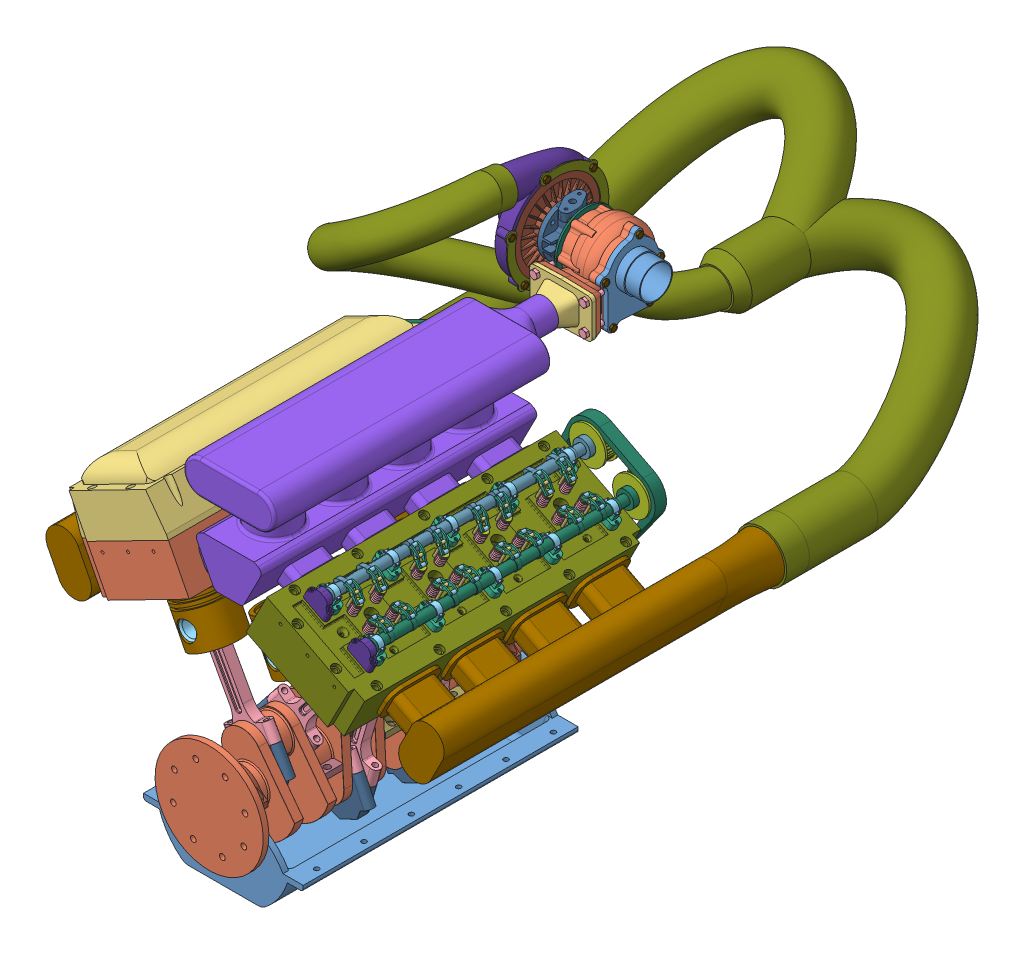
SolidWorks assembly ENSAMBLAJE DE MOTOR V8, configuration Predeterminado. Lengths in mm. (continued)
Mates (geometry in assembly coordinates): (continued)
- Distancia límite16: limit distance = 1.2344 mm: cone of assembly; cone of assembly; cone of CULATA_IZQUIERDO-2 through (128.2013 136.8296 302.75) axis (0.455744 0.890111 0); cone of VÁLVULA-18 through (127.4565 135.3748 302.75) axis (0.455744 0.890111 0)
- Concéntrica175: concentric: cylinder of assembly; cylinder of assembly; cylinder of CULATA_DERECHO-1 through (-129.9528 150.5383 696.25) axis (-0.455744 0.890111 0) radius 3; cylinder of VÁLVULA-1 through (-129.448 149.5524 696.25) axis (0.455744 -0.890111 0) radius 3
- Distancia límite13: limit distance = 0 mm: plane of assembly; plane of assembly; plane of CULATA_DERECHO-1 through (-140.7516 143.3241 454.25) normal (0.455744 -0.890111 0); plane of VÁLVULA-14 through (-155.9725 135.5309 434.25) normal (0.455744 -0.890111 0)
- Coincidente89: coincident: plane of assembly; plane of assembly; plane of RESORTE DE VÁLVULA-1 through (-174.795 238.1196 696.25) normal (-0.455744 0.890111 0); plane of VÁLVULA-1 through (-174.795 238.1196 696.25) normal (0.455744 -0.890111 0)
- Concéntrica176: concentric: cylinder of assembly; cylinder of assembly; cylinder of RESORTE DE VÁLVULA-1 through (-173.7217 236.0234 696.25) axis (-0.455744 0.890111 0) radius 7.3; cylinder of VÁLVULA-1 through (-129.448 149.5524 696.25) axis (0.455744 -0.890111 0) radius 3
- Distancia límite1: limit distance = 0.0087 mm: cone of assembly; cone of assembly; cone of CULATA_DERECHO-1 through (-129.9528 150.5383 696.25) axis (-0.455744 0.890111 0); cone of VÁLVULA-1 through (-129.2657 149.1964 696.25) axis (-0.455744 0.890111 0)
- Coincidente90: coincident: circle of CULATA_DERECHO-1; plane of ? through (-149.3077 210.2827 694) normal (0.455744 -0.890111 0)
- Concéntrica177: concentric: cylinder of CULATA_DERECHO-1 through (-156.1439 223.6343 696.25) axis (-0.455744 0.890111 0) radius 2.25; cylinder of ? through (-149.3077 210.2827 696.25) axis (0.455744 -0.890111 0) radius 2.25
- Paralelo3: parallel: plane of assembly; plane of assembly; plane of ARBOL DE LEVAS DE ADMISIÓN_DERECHO-1 through (-136.0099 236.5757 692.45) normal (0 0 -1); plane of EJE DE CONTROL DE VÁLVULAS-1 through (-180.6988 240.2228 703.25) normal (0 0 1)
- Paralelo4: parallel: plane of assembly; plane of assembly; plane of EJE DE CONTROL DE VÁLVULAS-1 through (-180.6988 240.2228 689.25) normal (0 0 -1); plane of RESORTE DE VÁLVULA-1 through (-160.667 210.5262 703.4) normal (0 0 1)
- Concéntrica178: concentric: cylinder of assembly; cylinder of assembly; cylinder of EJE DE CONTROL DE VÁLVULAS-1 through (-180.6988 240.2228 703.25) axis (0 0 -1) radius 2.5; cylinder of SOPORTE DE SEGUIDOR DE VÁLVULA-1 through (-180.6988 240.2228 691.95) axis (0 0 -1) radius 2.5
- Concéntrica179: concentric: cylinder of assembly; cylinder of assembly; cylinder of SOPORTE DE SEGUIDOR DE VÁLVULA-1 through (-191.9772 233.816 700.55) axis (0 0 -1) radius 1.9; cylinder of SEGUIDOR DE LEVA-13 through (-191.9772 233.816 700.05) axis (0 0 -1) radius 3
- Ancho17: width: plane of assembly; plane of assembly; plane of assembly; plane of assembly; plane of EJE DE CONTROL DE VÁLVULAS-1 through (-180.6988 240.2228 689.25) normal (0 0 -1); plane of EJE DE CONTROL DE VÁLVULAS-1 through (-180.6988 240.2228 703.25) normal (0 0 1); plane of SOPORTE DE SEGUIDOR DE VÁLVULA-1 through (-189.0856 245.1951 691.95) normal (0 0 1); plane of SOPORTE DE SEGUIDOR DE VÁLVULA-1 through (-176.0253 239.3734 700.55) normal (0 0 -1)
- Ancho18: width: plane of assembly; plane of assembly; plane of assembly; plane of assembly; plane of SOPORTE DE SEGUIDOR DE VÁLVULA-1 through (-176.0253 239.3734 700.55) normal (0 0 -1); plane of SOPORTE DE SEGUIDOR DE VÁLVULA-1 through (-189.0856 245.1951 691.95) normal (0 0 1); plane of SEGUIDOR DE LEVA-13 through (-191.9772 233.816 692.45) normal (0 0 -1); plane of SEGUIDOR DE LEVA-13 through (-191.9772 233.816 700.05) normal (0 0 1)
- Concéntrica181: concentric: cylinder of assembly; cylinder of assembly; cylinder of SEGUIDOR DE LEVA-1 through (-166.3151 243.7387 700.05) axis (0 0 -1) radius 3; cylinder of SOPORTE DE SEGUIDOR DE VÁLVULA-1 through (-166.3151 243.7387 700.55) axis (0 0 -1) radius 1.9
- Ancho19: width: plane of assembly; plane of assembly; plane of assembly; plane of assembly; plane of SOPORTE DE SEGUIDOR DE VÁLVULA-1 through (-189.0856 245.1951 689.45) normal (0 0 -1); plane of SOPORTE DE SEGUIDOR DE VÁLVULA-1 through (-176.0253 239.3734 703.05) normal (0 0 1); plane of SEGUIDOR DE LEVA-1 through (-166.3151 243.7387 700.05) normal (0 0 1); plane of SEGUIDOR DE LEVA-1 through (-166.3151 243.7387 692.45) normal (0 0 -1)
- Tangente3: tangent: plane of assembly; cylinder of assembly; plane of VÁLVULA-1 through (-175.2508 239.0097 696.25) normal (-0.455744 0.890111 0); cylinder of SEGUIDOR DE LEVA-13 through (-191.9772 233.816 700.05) axis (0 0 -1) radius 3
- Relación de posición de Leva Tangente1: cam tangent: cylinder of ARBOL DE LEVAS DE ADMISIÓN_DERECHO-1 through (-159.0489 247.0856 692.45) axis (0 0 1) radius 5; cylinder of SEGUIDOR DE LEVA-1 through (-166.3151 243.7387 700.05) axis (0 0 -1) radius 3
- Concéntrica182: concentric: cylinder of assembly; cylinder of assembly; cylinder of SOPORTE DE SEGUIDOR DE VÁLVULA-2 through (-177.5936 240.5206 588.55) axis (0 0 -1) radius 1.9; cylinder of SEGUIDOR DE LEVA-21 through (-177.5936 240.5206 588.05) axis (0 0 -1) radius 3
- Concéntrica183: concentric: cylinder of assembly; cylinder of assembly; cylinder of EJE DE CONTROL DE VÁLVULAS-2 through (-170.2719 251.2278 591.25) axis (0 0 -1) radius 2.5; cylinder of SOPORTE DE SEGUIDOR DE VÁLVULA-2 through (-170.2719 251.2278 579.95) axis (0 0 -1) radius 2.5
- Concéntrica184: concentric: cylinder of assembly; cylinder of assembly; cylinder of RESORTE DE VÁLVULA-2 through (-173.454 235.5005 584.25) axis (-0.455744 0.890111 0) radius 7.3; cylinder of VÁLVULA-2 through (-129.1802 149.0296 584.25) axis (0.455744 -0.890111 0) radius 3
- Ancho20: width: plane of SOPORTE DE SEGUIDOR DE VÁLVULA-2 through (-179.9902 252.0141 577.45) normal (0 0 -1); plane of SOPORTE DE SEGUIDOR DE VÁLVULA-2 through (-165.6999 252.5159 591.05) normal (0 0 1); plane of SEGUIDOR DE LEVA-17 through (-158.8913 260.7004 588.05) normal (0 0 1); plane of SEGUIDOR DE LEVA-17 through (-158.8913 260.7004 580.45) normal (0 0 -1)
- Ancho21: width: plane of assembly; plane of assembly; plane of assembly; plane of assembly; plane of EJE DE CONTROL DE VÁLVULAS-2 through (-170.2719 251.2278 577.25) normal (0 0 -1); plane of EJE DE CONTROL DE VÁLVULAS-2 through (-170.2719 251.2278 591.25) normal (0 0 1); plane of SOPORTE DE SEGUIDOR DE VÁLVULA-2 through (-179.9902 252.0141 579.95) normal (0 0 1); plane of SOPORTE DE SEGUIDOR DE VÁLVULA-2 through (-165.6999 252.5159 588.55) normal (0 0 -1)
- Concéntrica185: concentric: cylinder of SEGUIDOR DE LEVA-17 through (-158.8913 260.7004 588.05) axis (0 0 -1) radius 3; cylinder of SOPORTE DE SEGUIDOR DE VÁLVULA-2 through (-158.8913 260.7004 588.55) axis (0 0 -1) radius 1.9
- Tangente4: tangent: plane of assembly; cylinder of assembly; plane of VÁLVULA-2 through (-174.983 238.4868 584.25) normal (-0.455744 0.890111 0); cylinder of SEGUIDOR DE LEVA-21 through (-177.5936 240.5206 588.05) axis (0 0 -1) radius 3
- Paralelo5: parallel: plane of assembly; plane of assembly; plane of EJE DE CONTROL DE VÁLVULAS-2 through (-170.2719 251.2278 577.25) normal (0 0 -1); plane of RESORTE DE VÁLVULA-2 through (-160.3993 210.0033 591.4) normal (0 0 1)
- Ancho22: width: plane of assembly; plane of assembly; plane of assembly; plane of assembly; plane of SOPORTE DE SEGUIDOR DE VÁLVULA-2 through (-165.6999 252.5159 588.55) normal (0 0 -1); plane of SOPORTE DE SEGUIDOR DE VÁLVULA-2 through (-179.9902 252.0141 579.95) normal (0 0 1); plane of SEGUIDOR DE LEVA-21 through (-177.5936 240.5206 580.45) normal (0 0 -1); plane of SEGUIDOR DE LEVA-21 through (-177.5936 240.5206 588.05) normal (0 0 1)
- Coincidente93: coincident: plane of assembly; plane of assembly; plane of RESORTE DE VÁLVULA-2 through (-174.5273 237.5967 584.25) normal (-0.455744 0.890111 0); plane of VÁLVULA-2 through (-174.5273 237.5967 584.25) normal (0.455744 -0.890111 0)
- Coincidente94: coincident: circle of assembly; plane of assembly; circle of CULATA_DERECHO-1; plane of EJE DE CONTROL DE VÁLVULAS-2 through (-149.3077 210.2827 582) normal (0.455744 -0.890111 0)
- Concéntrica186: concentric: cylinder of assembly; cylinder of assembly; cylinder of CULATA_DERECHO-1 through (-129.9528 150.5383 584.25) axis (-0.455744 0.890111 0) radius 3; cylinder of VÁLVULA-2 through (-129.1802 149.0296 584.25) axis (0.455744 -0.890111 0) radius 3
- Distancia límite2: limit distance = 1.6951 mm: plane of assembly; plane of assembly; plane of CULATA_DERECHO-1 through (-140.7516 143.3241 564.25) normal (0.455744 -0.890111 0); plane of VÁLVULA-2 through (-128.4966 147.6944 584.25) normal (0.455744 -0.890111 0)
- Concéntrica187: concentric: cylinder of assembly; cylinder of assembly; cylinder of CULATA_DERECHO-1 through (-156.1439 223.6343 584.25) axis (-0.455744 0.890111 0) radius 2.25; cylinder of EJE DE CONTROL DE VÁLVULAS-2 through (-149.3077 210.2827 584.25) axis (0.455744 -0.890111 0) radius 2.25
- Paralelo6: parallel: plane of assembly; plane of assembly; plane of RESORTE DE VÁLVULA-2 through (-160.3993 210.0033 577.1) normal (0 0 -1); plane of SOPORTE DE SEGUIDOR DE VÁLVULA-2 through (-179.9902 252.0141 577.45) normal (0 0 -1)
- Relación de posición de Leva Tangente2: cam tangent: cylinder of ARBOL DE LEVAS DE ADMISIÓN_DERECHO-1 through (-150.1483 251.4202 588.05) axis (0 0 -1) radius 9.75; cylinder of SEGUIDOR DE LEVA-17 through (-158.8913 260.7004 588.05) axis (0 0 -1) radius 3
- Paralelo9: parallel: plane of assembly; plane of assembly; plane of ARBOL DE LEVAS DE ADMISIÓN_DERECHO-1 through (-170.2396 250.2568 588.05) normal (0 0 1); plane of SOPORTE DE SEGUIDOR DE VÁLVULA-2 through (-165.6999 252.5159 591.05) normal (0 0 1)
- Distancia límite4: limit distance = 1.1076 mm: plane of assembly; plane of assembly; plane of CULATA_DERECHO-1 through (-140.7516 143.3241 676.25) normal (0.455744 -0.890111 0); plane of VÁLVULA-3 through (-128.7643 148.2172 656.25) normal (0.455744 -0.890111 0)
- Distancia límite5: limit distance = 1.6951 mm: plane of assembly; plane of assembly; plane of CULATA_DERECHO-1 through (-140.7516 143.3241 564.25) normal (0.455744 -0.890111 0); plane of VÁLVULA-4 through (-128.4966 147.6944 544.25) normal (0.455744 -0.890111 0)
- Distancia límite6: limit distance = 1.1076 mm: plane of assembly; plane of assembly; plane of CULATA_DERECHO-1 through (-140.7516 143.3241 344.25) normal (0.455744 -0.890111 0); plane of VÁLVULA-6 through (-128.7643 148.2172 324.25) normal (0.455744 -0.890111 0)
- Distancia límite7: limit distance = 1.1076 mm: plane of assembly; plane of assembly; plane of CULATA_DERECHO-1 through (-140.7516 143.3241 344.25) normal (0.455744 -0.890111 0); plane of VÁLVULA-5 through (-128.7643 148.2172 364.25) normal (0.455744 -0.890111 0)
- Concéntrica189: concentric: cylinder of assembly; cylinder of assembly; cylinder of RESORTE DE VÁLVULA-9 through (-200.4251 222.3511 696.25) axis (-0.455744 0.890111 0) radius 7.3; cylinder of VÁLVULA-9 through (-156.1513 135.8801 696.25) axis (0.455744 -0.890111 0) radius 3
- Coincidente96: coincident: plane of RESORTE DE VÁLVULA-9 through (-201.4983 224.4473 696.25) normal (-0.455744 0.890111 0); plane of VÁLVULA-9 through (-201.4983 224.4473 696.25) normal (0.455744 -0.890111 0)
- Concéntrica190: concentric: cylinder of CULATA_DERECHO-1 through (-156.6561 136.866 696.25) axis (-0.455744 0.890111 0) radius 3; cylinder of VÁLVULA-9 through (-156.1513 135.8801 696.25) axis (0.455744 -0.890111 0) radius 3
- Distancia límite8: limit distance = 1.1076 mm: plane of CULATA_DERECHO-1 through (-140.7516 143.3241 676.25) normal (0.455744 -0.890111 0); plane of VÁLVULA-9 through (-155.4677 134.5449 696.25) normal (0.455744 -0.890111 0)
- Concéntrica191: concentric: cylinder of assembly; cylinder of assembly; cylinder of EJE DE CONTROL DE VÁLVULAS-9 through (-214.7775 228.4406 689.25) axis (0 0 1) radius 2.5; cylinder of SOPORTE DE SEGUIDOR DE VÁLVULA-9 through (-214.7775 228.4406 700.55) axis (0 0 1) radius 2.5
- Concéntrica192: concentric: cylinder of SEGUIDOR DE LEVA-25 through (-201.8109 228.7811 692.45) axis (0 0 1) radius 3; cylinder of SOPORTE DE SEGUIDOR DE VÁLVULA-9 through (-201.8109 228.7811 691.95) axis (0 0 1) radius 1.9
- Concéntrica193: concentric: cylinder of SOPORTE DE SEGUIDOR DE VÁLVULA-9 through (-228.9095 224.0206 691.95) axis (0 0 1) radius 1.9; cylinder of SEGUIDOR DE LEVA-34 through (-228.9095 224.0206 692.45) axis (0 0 1) radius 3
- Ancho24: width: plane of SOPORTE DE SEGUIDOR DE VÁLVULA-9 through (-210.1649 237.0305 703.05) normal (0 0 1); plane of SOPORTE DE SEGUIDOR DE VÁLVULA-9 through (-218.3403 225.299 689.45) normal (0 0 -1); plane of SEGUIDOR DE LEVA-34 through (-228.9095 224.0206 692.45) normal (0 0 -1); plane of SEGUIDOR DE LEVA-34 through (-228.9095 224.0206 700.05) normal (0 0 1)
- Ancho25: width: plane of SOPORTE DE SEGUIDOR DE VÁLVULA-9 through (-210.1649 237.0305 703.05) normal (0 0 1); plane of SOPORTE DE SEGUIDOR DE VÁLVULA-9 through (-218.3403 225.299 689.45) normal (0 0 -1); plane of EJE DE CONTROL DE VÁLVULAS-9 through (-214.7775 228.4406 703.25) normal (0 0 1); plane of EJE DE CONTROL DE VÁLVULAS-9 through (-214.7775 228.4406 689.25) normal (0 0 -1)
- Ancho26: width: plane of SEGUIDOR DE LEVA-25 through (-201.8109 228.7811 700.05) normal (0 0 1); plane of SEGUIDOR DE LEVA-25 through (-201.8109 228.7811 692.45) normal (0 0 -1); plane of SOPORTE DE SEGUIDOR DE VÁLVULA-9 through (-218.3403 225.299 689.45) normal (0 0 -1); plane of SOPORTE DE SEGUIDOR DE VÁLVULA-9 through (-210.1649 237.0305 703.05) normal (0 0 1)
- Concéntrica194: concentric: cylinder of assembly; cylinder of assembly; cylinder of RESORTE DE VÁLVULA-10 through (-190.6415 203.2427 584.25) axis (-0.455744 0.890111 0) radius 5.25; cylinder of VÁLVULA-10 through (-156.6561 136.866 584.25) axis (0.455744 -0.890111 0) radius 3
- Concéntrica195: concentric: cylinder of assembly; cylinder of assembly; cylinder of SEGUIDOR DE LEVA-38 through (-228.4393 222.7305 580.45) axis (0 0 1) radius 3; cylinder of SOPORTE DE SEGUIDOR DE VÁLVULA-10 through (-228.4393 222.7305 579.95) axis (0 0 1) radius 1.9
- Concéntrica196: concentric: cylinder of EJE DE CONTROL DE VÁLVULAS-10 through (-214.7775 228.4406 591.25) axis (0 0 -1) radius 2.5; cylinder of SOPORTE DE SEGUIDOR DE VÁLVULA-10 through (-214.7775 228.4406 577.45) axis (0 0 1) radius 2.5
- Concéntrica197: concentric: cylinder of CULATA_DERECHO-1 through (-200.6495 200.8471 584.25) axis (-0.455744 0.890111 0) radius 2.25; cylinder of EJE DE CONTROL DE VÁLVULAS-10 through (-193.8133 187.4955 584.25) axis (0.455744 -0.890111 0) radius 2.25
- Ancho27: width: plane of SOPORTE DE SEGUIDOR DE VÁLVULA-10 through (-210.9805 237.4209 588.55) normal (0 0 -1); plane of SOPORTE DE SEGUIDOR DE VÁLVULA-10 through (-218.0339 224.9825 579.95) normal (0 0 1); plane of EJE DE CONTROL DE VÁLVULAS-10 through (-214.7775 228.4406 591.25) normal (0 0 1); plane of EJE DE CONTROL DE VÁLVULAS-10 through (-214.7775 228.4406 577.25) normal (0 0 -1)
- Coincidente100: coincident: circle of CULATA_DERECHO-1; plane of EJE DE CONTROL DE VÁLVULAS-10 through (-193.8133 187.4955 582) normal (0.455744 -0.890111 0)
- Ancho28: width: plane of ARBOL DE LEVAS DE ESCAPE_DERECHO-1 through (-245.4839 205.0082 580.45) normal (0 0 -1); plane of ARBOL DE LEVAS DE ESCAPE_DERECHO-1 through (-245.4839 205.0082 588.05) normal (0 0 1); plane of EJE DE CONTROL DE VÁLVULAS-10 through (-214.7775 228.4406 591.25) normal (0 0 1); plane of EJE DE CONTROL DE VÁLVULAS-10 through (-214.7775 228.4406 577.25) normal (0 0 -1)
- Ancho29: width: plane of SEGUIDOR DE LEVA-38 through (-228.4393 222.7305 588.05) normal (0 0 1); plane of SEGUIDOR DE LEVA-38 through (-228.4393 222.7305 580.45) normal (0 0 -1); plane of SOPORTE DE SEGUIDOR DE VÁLVULA-10 through (-218.0339 224.9825 577.45) normal (0 0 -1); plane of SOPORTE DE SEGUIDOR DE VÁLVULA-10 through (-210.9805 237.4209 591.05) normal (0 0 1)
- Concéntrica198: concentric: cylinder of assembly; cylinder of assembly; cylinder of CULATA_DERECHO-1 through (-187.1909 196.5035 584.25) axis (-0.455744 0.890111 0) radius 7.3; cylinder of VÁLVULA-10 through (-156.6561 136.866 584.25) axis (0.455744 -0.890111 0) radius 3
- Coincidente101: coincident: plane of RESORTE DE VÁLVULA-10 through (-202.0031 225.4332 584.25) normal (-0.455744 0.890111 0); plane of VÁLVULA-10 through (-202.0031 225.4332 584.25) normal (0.455744 -0.890111 0)
- Concéntrica199: concentric: cylinder of SOPORTE DE SEGUIDOR DE VÁLVULA-10 through (-201.8981 229.9808 579.95) axis (0 0 1) radius 1.9; cylinder of SEGUIDOR DE LEVA-42 through (-201.8981 229.9808 588.05) axis (0 0 -1) radius 1.9
- Ancho30: width: plane of SEGUIDOR DE LEVA-42 through (-201.8981 229.9808 588.05) normal (0 0 1); plane of SEGUIDOR DE LEVA-42 through (-201.8981 229.9808 580.45) normal (0 0 -1); plane of SOPORTE DE SEGUIDOR DE VÁLVULA-10 through (-210.9805 237.4209 591.05) normal (0 0 1); plane of SOPORTE DE SEGUIDOR DE VÁLVULA-10 through (-218.0339 224.9825 577.45) normal (0 0 -1)
- Tangente6: tangent: plane of VÁLVULA-10 through (-202.4589 226.3233 584.25) normal (-0.455744 0.890111 0); cylinder of SEGUIDOR DE LEVA-42 through (-201.8981 229.9808 588.05) axis (0 0 -1) radius 3
- Distancia límite10: limit distance = 1.1076 mm: plane of assembly; plane of assembly; plane of CULATA_DERECHO-1 through (-140.7516 143.3241 676.25) normal (0.455744 -0.890111 0); plane of VÁLVULA-11 through (-155.4677 134.5449 656.25) normal (0.455744 -0.890111 0)
- Distancia límite14: limit distance = 1.1076 mm: plane of assembly; plane of assembly; plane of CULATA_DERECHO-1 through (-140.7516 143.3241 344.25) normal (0.455744 -0.890111 0); plane of VÁLVULA-15 through (-155.4677 134.5449 364.25) normal (0.455744 -0.890111 0)
- Distancia límite15: limit distance = 1.1076 mm: plane of assembly; plane of assembly; plane of CULATA_DERECHO-1 through (-140.7516 143.3241 344.25) normal (0.455744 -0.890111 0); plane of VÁLVULA-16 through (-155.4677 134.5449 324.25) normal (0.455744 -0.890111 0)
- Concéntrica201: concentric: cylinder of assembly; cylinder of assembly; cylinder of CULATA_IZQUIERDO-2 through (172.1947 200.8107 302.75) axis (0.455744 0.890111 0) radius 2.25; cylinder of EJE DE CONTROL DE VÁLVULAS-17 through (165.3585 187.459 302.75) axis (-0.455744 -0.890111 0) radius 2.25
- Concéntrica202: concentric: cylinder of assembly; cylinder of assembly; cylinder of RESORTE DE VÁLVULA-17 through (161.6241 202.1075 302.75) axis (0.455744 0.890111 0) radius 5.25; cylinder of VÁLVULA-18 through (127.6388 135.7308 302.75) axis (-0.455744 -0.890111 0) radius 3
- Coincidente103: coincident: plane of RESORTE DE VÁLVULA-17 through (172.9858 224.298 302.75) normal (0.455744 0.890111 0); plane of VÁLVULA-18 through (172.9858 224.298 302.75) normal (-0.455744 -0.890111 0)
- Concéntrica203: concentric: cylinder of assembly; cylinder of assembly; cylinder of CULATA_IZQUIERDO-2 through (128.2013 136.8296 302.75) axis (0.455744 0.890111 0) radius 3; cylinder of VÁLVULA-18 through (127.6388 135.7308 302.75) axis (-0.455744 -0.890111 0) radius 3
- Concéntrica204: concentric: cylinder of assembly; cylinder of assembly; cylinder of SEGUIDOR DE LEVA-46 through (200.5019 224.138 306.55) axis (0 0 -1) radius 3; cylinder of SOPORTE DE SEGUIDOR DE VÁLVULA-19 through (200.5019 224.138 307.05) axis (0 0 -1) radius 1.9
- Concéntrica205: concentric: cylinder of EJE DE CONTROL DE VÁLVULAS-17 through (186.3227 228.4041 309.75) axis (0 0 -1) radius 2.5; cylinder of SOPORTE DE SEGUIDOR DE VÁLVULA-19 through (186.3227 228.4041 309.55) axis (0 0 -1) radius 2.5
- Ancho33: width: plane of SOPORTE DE SEGUIDOR DE VÁLVULA-19 through (181.6171 236.9434 295.95) normal (0 0 -1); plane of SOPORTE DE SEGUIDOR DE VÁLVULA-19 through (189.9194 225.3015 309.55) normal (0 0 1); plane of EJE DE CONTROL DE VÁLVULAS-17 through (186.3227 228.4041 309.75) normal (0 0 1); plane of EJE DE CONTROL DE VÁLVULAS-17 through (186.3227 228.4041 295.75) normal (0 0 -1)
- Concéntrica206: concentric: cylinder of SOPORTE DE SEGUIDOR DE VÁLVULA-19 through (173.3532 228.6038 307.05) axis (0 0 -1) radius 1.9; cylinder of SEGUIDOR DE LEVA-53 through (173.3532 228.6038 306.55) axis (0 0 -1) radius 3
- Ancho34: width: plane of SOPORTE DE SEGUIDOR DE VÁLVULA-19 through (181.6171 236.9434 295.95) normal (0 0 -1); plane of SOPORTE DE SEGUIDOR DE VÁLVULA-19 through (189.9194 225.3015 309.55) normal (0 0 1); plane of SEGUIDOR DE LEVA-53 through (173.3532 228.6038 306.55) normal (0 0 1); plane of SEGUIDOR DE LEVA-53 through (173.3532 228.6038 298.95) normal (0 0 -1)
- Tangente7: tangent: plane of VÁLVULA-18 through (173.4416 225.1881 302.75) normal (0.455744 0.890111 0); cylinder of SEGUIDOR DE LEVA-53 through (173.3532 228.6038 306.55) axis (0 0 -1) radius 3
- Concéntrica210: concentric: cylinder of RESORTE DE VÁLVULA-19 through (161.4142 201.6975 412.75) axis (0.455744 0.890111 0) radius 5.25; cylinder of ? through (127.4288 135.3208 412.75) axis (-0.455744 -0.890111 0) radius 3
- Concéntrica211: concentric: cylinder of assembly; cylinder of assembly; cylinder of SEGUIDOR DE LEVA-57 through (200.6612 224.7083 416.55) axis (0 0 -1) radius 3; cylinder of SOPORTE DE SEGUIDOR DE VÁLVULA-21 through (200.6612 224.7083 417.05) axis (0 0 -1) radius 1.9
- Concéntrica212: concentric: cylinder of EJE DE CONTROL DE VÁLVULAS-19 through (186.3227 228.4041 405.75) axis (0 0 1) radius 2.5; cylinder of SOPORTE DE SEGUIDOR DE VÁLVULA-21 through (186.3227 228.4041 419.55) axis (0 0 -1) radius 2.5
- Ancho35: width: plane of SOPORTE DE SEGUIDOR DE VÁLVULA-21 through (181.2794 236.7485 405.95) normal (0 0 -1); plane of SOPORTE DE SEGUIDOR DE VÁLVULA-21 through (190.0406 225.4478 419.55) normal (0 0 1); plane of EJE DE CONTROL DE VÁLVULAS-19 through (186.3227 228.4041 419.75) normal (0 0 1); plane of EJE DE CONTROL DE VÁLVULAS-19 through (186.3227 228.4041 405.75) normal (0 0 -1)
- Coincidente106: coincident: plane of CULATA_IZQUIERDO-2 through (165.3585 187.459 410.5) normal (0.455744 0.890111 0); plane of EJE DE CONTROL DE VÁLVULAS-19 through (165.3585 187.459 415) normal (-0.455744 -0.890111 0)
- Concéntrica214: concentric: cylinder of SEGUIDOR DE LEVA-57 through (200.6612 224.7083 416.55) axis (0 0 -1) radius 3; cylinder of SOPORTE DE SEGUIDOR DE VÁLVULA-21 through (200.6612 224.7083 417.05) axis (0 0 -1) radius 1.9
- Ancho36: width: plane of SOPORTE DE SEGUIDOR DE VÁLVULA-21 through (190.0406 225.4478 419.55) normal (0 0 1); plane of SOPORTE DE SEGUIDOR DE VÁLVULA-21 through (181.2794 236.7485 405.95) normal (0 0 -1); plane of SEGUIDOR DE LEVA-57 through (200.6612 224.7083 408.95) normal (0 0 -1); plane of SEGUIDOR DE LEVA-57 through (200.6612 224.7083 416.55) normal (0 0 1)
- Concéntrica215: concentric: cylinder of CULATA_IZQUIERDO-2 through (158.7361 196.467 412.75) axis (0.455744 0.890111 0) radius 7.3; cylinder of ? through (127.4288 135.3208 412.75) axis (-0.455744 -0.890111 0) radius 3
- Coincidente107: coincident: plane of RESORTE DE VÁLVULA-19 through (172.7759 223.888 412.75) normal (0.455744 0.890111 0); plane of ? through (172.7759 223.888 412.75) normal (-0.455744 -0.890111 0)
- Distancia límite17: limit distance = 1.6951 mm: cylinder of CULATA_IZQUIERDO-2 through (128.2013 136.8296 412.75) axis (0.455744 0.890111 0) radius 1421.9064; cylinder of ? through (127.2465 134.9647 412.75) axis (0.455744 0.890111 0) radius 1420.7568
- Relación de posición de Leva Tangente7: cam tangent: cylinder of ARBOL DE LEVAS DE ESCAPE_IZQUIERDO-2 through (236.8793 200.9068 416.55) axis (0 0 -1) radius 50; cylinder of SEGUIDOR DE LEVA-57 through (200.6612 224.7083 416.55) axis (0 0 -1) radius 3
- Concéntrica216: concentric: cylinder of SOPORTE DE SEGUIDOR DE VÁLVULA-21 through (173.3555 228.085 417.05) axis (0 0 -1) radius 1.9; cylinder of SEGUIDOR DE LEVA-61 through (173.3555 228.085 416.55) axis (0 0 -1) radius 3
- Ancho37: width: plane of SEGUIDOR DE LEVA-61 through (173.3555 228.085 408.95) normal (0 0 -1); plane of SEGUIDOR DE LEVA-61 through (173.3555 228.085 416.55) normal (0 0 1); plane of SOPORTE DE SEGUIDOR DE VÁLVULA-21 through (190.0406 225.4478 417.05) normal (0 0 -1); plane of SOPORTE DE SEGUIDOR DE VÁLVULA-21 through (181.2794 236.7485 408.45) normal (0 0 1)
- Tangente9: tangent: plane of ? through (173.2316 224.7781 412.75) normal (0.455744 0.890111 0); cylinder of SEGUIDOR DE LEVA-61 through (173.3555 228.085 416.55) axis (0 0 -1) radius 3
- Distancia límite18: limit distance = 1.2344 mm: plane of assembly; plane of assembly; plane of CULATA_IZQUIERDO-2 through (112.2968 143.2876 322.75) normal (-0.455744 -0.890111 0); plane of VÁLVULA-21 through (126.9551 134.3957 342.75) normal (-0.455744 -0.890111 0)
- Distancia límite19: limit distance = 1.6951 mm: plane of CULATA_IZQUIERDO-2 through (112.2968 143.2876 432.75) normal (-0.455744 -0.890111 0); plane of ? through (126.7452 133.9856 452.75) normal (-0.455744 -0.890111 0)
- Distancia límite21: limit distance = 1.6951 mm: plane of CULATA_IZQUIERDO-2 through (112.2968 143.2876 542.75) normal (-0.455744 -0.890111 0); plane of ? through (126.7452 133.9856 562.75) normal (-0.455744 -0.890111 0)
- Distancia límite22: limit distance = 1.2344 mm: plane of assembly; plane of assembly; plane of CULATA_IZQUIERDO-2 through (112.2968 143.2876 654.75) normal (-0.455744 -0.890111 0); plane of VÁLVULA-25 through (126.9551 134.3957 634.75) normal (-0.455744 -0.890111 0)
- Distancia límite23: limit distance = 1.2344 mm: plane of assembly; plane of assembly; plane of CULATA_IZQUIERDO-2 through (112.2968 143.2876 654.75) normal (-0.455744 -0.890111 0); plane of VÁLVULA-26 through (126.9551 134.3957 674.75) normal (-0.455744 -0.890111 0)
- Concéntrica217: concentric: cylinder of assembly; cylinder of assembly; cylinder of EJE DE CONTROL DE VÁLVULAS-26 through (141.8172 251.1913 681.75) axis (0 0 -1) radius 2.5; cylinder of SOPORTE DE SEGUIDOR DE VÁLVULA-28 through (141.8172 251.1913 679.05) axis (0 0 1) radius 2.5
- Concéntrica218: concentric: cylinder of assembly; cylinder of assembly; cylinder of RESORTE DE VÁLVULA-26 through (134.9786 215.8927 674.75) axis (0.455744 0.890111 0) radius 5.25; cylinder of VÁLVULA-27 through (100.9932 149.516 674.75) axis (-0.455744 -0.890111 0) radius 3
- Concéntrica219: concentric: cylinder of SEGUIDOR DE LEVA-65 through (129.9696 260.0731 670.95) axis (0 0 1) radius 3; cylinder of SOPORTE DE SEGUIDOR DE VÁLVULA-28 through (129.9696 260.0731 670.45) axis (0 0 1) radius 1.9
- Coincidente108: coincident: plane of RESORTE DE VÁLVULA-26 through (146.3402 238.0831 674.75) normal (0.455744 0.890111 0); plane of VÁLVULA-27 through (146.3402 238.0831 674.75) normal (-0.455744 -0.890111 0)
- Ancho38: width: plane of EJE DE CONTROL DE VÁLVULAS-26 through (141.8172 251.1913 667.75) normal (0 0 -1); plane of EJE DE CONTROL DE VÁLVULAS-26 through (141.8172 251.1913 681.75) normal (0 0 1); plane of SOPORTE DE SEGUIDOR DE VÁLVULA-28 through (151.4829 252.4707 681.55) normal (0 0 1); plane of SOPORTE DE SEGUIDOR DE VÁLVULA-28 through (137.1856 252.2453 667.95) normal (0 0 -1)
- Ancho39: width: plane of SOPORTE DE SEGUIDOR DE VÁLVULA-28 through (137.1856 252.2453 667.95) normal (0 0 -1); plane of SOPORTE DE SEGUIDOR DE VÁLVULA-28 through (151.4829 252.4707 681.55) normal (0 0 1); plane of SEGUIDOR DE LEVA-65 through (129.9696 260.0731 678.55) normal (0 0 1); plane of SEGUIDOR DE LEVA-65 through (129.9696 260.0731 670.95) normal (0 0 -1)
- Concéntrica220: concentric: cylinder of CULATA_IZQUIERDO-2 through (101.498 150.5019 674.75) axis (0.455744 0.890111 0) radius 3; cylinder of VÁLVULA-27 through (100.9932 149.516 674.75) axis (-0.455744 -0.890111 0) radius 3
- Distancia límite24: limit distance = 1.1076 mm: plane of CULATA_IZQUIERDO-2 through (112.2968 143.2876 654.75) normal (-0.455744 -0.890111 0); plane of VÁLVULA-27 through (100.3096 148.1808 674.75) normal (-0.455744 -0.890111 0)
- Concéntrica221: concentric: cylinder of CULATA_IZQUIERDO-2 through (127.6891 223.5979 674.75) axis (0.455744 0.890111 0) radius 2.25; cylinder of EJE DE CONTROL DE VÁLVULAS-26 through (120.853 210.2462 674.75) axis (-0.455744 -0.890111 0) radius 2.25
- Coincidente110: coincident: circle of CULATA_IZQUIERDO-2; plane of EJE DE CONTROL DE VÁLVULAS-26 through (120.853 210.2462 672.5) normal (-0.455744 -0.890111 0)
- Ancho40: width: plane of SOPORTE DE SEGUIDOR DE VÁLVULA-28 through (137.1856 252.2453 667.95) normal (0 0 -1); plane of SOPORTE DE SEGUIDOR DE VÁLVULA-28 through (151.4829 252.4707 681.55) normal (0 0 1); plane of ARBOL DE LEVAS DE ADMISIÓN_IZQUIERDO-2 through (133.1776 268.365 670.95) normal (0 0 -1); plane of ARBOL DE LEVAS DE ADMISIÓN_IZQUIERDO-2 through (133.1776 268.365 678.55) normal (0 0 1)
- Relación de posición de Leva Tangente8: cam tangent: cylinder of ARBOL DE LEVAS DE ADMISIÓN_IZQUIERDO-2 through (144.6617 285.3463 670.95) axis (0 0 1) radius 50; cylinder of SEGUIDOR DE LEVA-65 through (129.9696 260.0731 670.95) axis (0 0 1) radius 3
- Concéntrica222: concentric: cylinder of SOPORTE DE SEGUIDOR DE VÁLVULA-28 through (149.6737 240.8702 670.45) axis (0 0 1) radius 1.9; cylinder of SEGUIDOR DE LEVA-69 through (149.6737 240.8702 678.55) axis (0 0 -1) radius 3
- Ancho41: width: plane of SEGUIDOR DE LEVA-69 through (149.6737 240.8702 678.55) normal (0 0 1); plane of SEGUIDOR DE LEVA-69 through (149.6737 240.8702 670.95) normal (0 0 -1); plane of SOPORTE DE SEGUIDOR DE VÁLVULA-28 through (137.1856 252.2453 667.95) normal (0 0 -1); plane of SOPORTE DE SEGUIDOR DE VÁLVULA-28 through (151.4829 252.4707 681.55) normal (0 0 1)
- Tangente11: tangent: plane of VÁLVULA-27 through (146.796 238.9732 674.75) normal (0.455744 0.890111 0); cylinder of SEGUIDOR DE LEVA-69 through (149.6737 240.8702 678.55) axis (0 0 -1) radius 3
- Concéntrica223: concentric: cylinder of assembly; cylinder of assembly; cylinder of EJE DE CONTROL DE VÁLVULAS-27 through (141.8172 251.1913 569.75) axis (0 0 -1) radius 2.5; cylinder of SOPORTE DE SEGUIDOR DE VÁLVULA-29 through (141.8172 251.1913 555.95) axis (0 0 1) radius 2.5
- Concéntrica224: concentric: cylinder of SEGUIDOR DE LEVA-73 through (147.0712 239.3319 558.95) axis (0 0 1) radius 1.9; cylinder of SOPORTE DE SEGUIDOR DE VÁLVULA-29 through (147.0712 239.3319 558.45) axis (0 0 1) radius 1.9
- Concéntrica225: concentric: cylinder of assembly; cylinder of assembly; cylinder of RESORTE DE VÁLVULA-27 through (133.814 213.6181 562.75) axis (0.455744 0.890111 0) radius 5.25; cylinder of VÁLVULA-28 through (99.8286 147.2414 562.75) axis (-0.455744 -0.890111 0) radius 3
- Coincidente111: coincident: plane of RESORTE DE VÁLVULA-27 through (145.1757 235.8086 562.75) normal (0.455744 0.890111 0); plane of VÁLVULA-28 through (145.1757 235.8086 562.75) normal (-0.455744 -0.890111 0)
- Ancho42: width: plane of EJE DE CONTROL DE VÁLVULAS-27 through (141.8172 251.1913 555.75) normal (0 0 -1); plane of EJE DE CONTROL DE VÁLVULAS-27 through (141.8172 251.1913 569.75) normal (0 0 1); plane of SOPORTE DE SEGUIDOR DE VÁLVULA-29 through (151.5165 250.1985 569.55) normal (0 0 1); plane of SOPORTE DE SEGUIDOR DE VÁLVULA-29 through (137.5554 253.2888 555.95) normal (0 0 -1)
- Ancho43: width: plane of SEGUIDOR DE LEVA-73 through (147.0712 239.3319 558.95) normal (0 0 -1); plane of SEGUIDOR DE LEVA-73 through (147.0712 239.3319 566.55) normal (0 0 1); plane of SOPORTE DE SEGUIDOR DE VÁLVULA-29 through (151.5165 250.1985 569.55) normal (0 0 1); plane of SOPORTE DE SEGUIDOR DE VÁLVULA-29 through (137.5554 253.2888 555.95) normal (0 0 -1)
- Coincidente112: coincident: circle of CULATA_IZQUIERDO-2; plane of EJE DE CONTROL DE VÁLVULAS-27 through (120.853 210.2462 560.5) normal (-0.455744 -0.890111 0)
- Concéntrica226: concentric: cylinder of CULATA_IZQUIERDO-2 through (127.6891 223.5979 562.75) axis (0.455744 0.890111 0) radius 2.25; cylinder of EJE DE CONTROL DE VÁLVULAS-27 through (120.853 210.2462 562.75) axis (-0.455744 -0.890111 0) radius 2.25
- Ancho44: width: plane of SOPORTE DE SEGUIDOR DE VÁLVULA-29 through (151.5165 250.1985 569.55) normal (0 0 1); plane of SOPORTE DE SEGUIDOR DE VÁLVULA-29 through (137.5554 253.2888 555.95) normal (0 0 -1); plane of ARBOL DE LEVAS DE ADMISIÓN_IZQUIERDO-2 through (101.687 249.2029 566.55) normal (0 0 1); plane of ARBOL DE LEVAS DE ADMISIÓN_IZQUIERDO-2 through (101.687 249.2029 558.95) normal (0 0 -1)
- Concéntrica227: concentric: cylinder of CULATA_IZQUIERDO-2 through (132.0328 210.1393 562.75) axis (0.455744 0.890111 0) radius 7.3; cylinder of VÁLVULA-28 through (99.8286 147.2414 562.75) axis (-0.455744 -0.890111 0) radius 3
- Distancia límite25: limit distance = 3.663 mm: plane of CULATA_IZQUIERDO-2 through (112.2968 143.2876 542.75) normal (-0.455744 -0.890111 0); plane of VÁLVULA-28 through (99.145 145.9063 562.75) normal (-0.455744 -0.890111 0)
- Tangente12: tangent: cylinder of SEGUIDOR DE LEVA-73 through (147.0712 239.3319 558.95) axis (0 0 1) radius 3; plane of VÁLVULA-28 through (145.6314 236.6987 562.75) normal (0.455744 0.890111 0)
- Concéntrica228: concentric: cylinder of SOPORTE DE SEGUIDOR DE VÁLVULA-29 through (132.3474 262.5743 558.45) axis (0 0 1) radius 1.9; cylinder of SEGUIDOR DE LEVA-77 through (132.3474 262.5743 566.55) axis (0 0 -1) radius 1.9
- Ancho45: width: plane of SEGUIDOR DE LEVA-77 through (132.3474 262.5743 566.55) normal (0 0 1); plane of SEGUIDOR DE LEVA-77 through (132.3474 262.5743 558.95) normal (0 0 -1); plane of SOPORTE DE SEGUIDOR DE VÁLVULA-29 through (137.5554 253.2888 555.95) normal (0 0 -1); plane of SOPORTE DE SEGUIDOR DE VÁLVULA-29 through (151.5165 250.1985 569.55) normal (0 0 1)
- Relación de posición de Leva Tangente10: cam tangent: cylinder of ARBOL DE LEVAS DE ADMISIÓN_IZQUIERDO-2 through (152.9371 226.0086 566.55) axis (0 0 -1) radius 50; cylinder of SEGUIDOR DE LEVA-77 through (132.3474 262.5743 566.55) axis (0 0 -1) radius 3
- Paralelo18: parallel: plane of SOPORTE DE SEGUIDOR DE VÁLVULA-21 through (181.2794 236.7485 405.95) normal (0 0 -1); plane of RESORTE DE VÁLVULA-19 through (158.6478 196.2945 405.6) normal (0 0 -1)
- Distancia límite26: limit distance = 1.1076 mm: plane of assembly; plane of assembly; plane of CULATA_IZQUIERDO-2 through (112.2968 143.2876 654.75) normal (-0.455744 -0.890111 0); plane of VÁLVULA-29 through (100.3096 148.1808 634.75) normal (-0.455744 -0.890111 0)
- Distancia límite27: limit distance = 3.663 mm: plane of assembly; plane of assembly; plane of CULATA_IZQUIERDO-2 through (112.2968 143.2876 542.75) normal (-0.455744 -0.890111 0); plane of VÁLVULA-30 through (99.145 145.9063 522.75) normal (-0.455744 -0.890111 0)
- Distancia límite28: limit distance = 3.663 mm: plane of assembly; plane of assembly; plane of CULATA_IZQUIERDO-2 through (112.2968 143.2876 432.75) normal (-0.455744 -0.890111 0); plane of VÁLVULA-31 through (99.145 145.9063 452.75) normal (-0.455744 -0.890111 0)
- Distancia límite29: limit distance = 3.663 mm: plane of assembly; plane of assembly; plane of CULATA_IZQUIERDO-2 through (112.2968 143.2876 432.75) normal (-0.455744 -0.890111 0); plane of VÁLVULA-32 through (99.145 145.9063 412.75) normal (-0.455744 -0.890111 0)
- Distancia límite30: limit distance = 1.1076 mm: plane of assembly; plane of assembly; plane of CULATA_IZQUIERDO-2 through (112.2968 143.2876 322.75) normal (-0.455744 -0.890111 0); plane of VÁLVULA-33 through (100.3096 148.1808 342.75) normal (-0.455744 -0.890111 0)
- Distancia límite31: limit distance = 1.1076 mm: plane of assembly; plane of assembly; plane of CULATA_IZQUIERDO-2 through (112.2968 143.2876 322.75) normal (-0.455744 -0.890111 0); plane of VÁLVULA-34 through (100.3096 148.1808 302.75) normal (-0.455744 -0.890111 0)
- Concéntrica229: concentric: cylinder of ? through (-14.263 -103.8973 740.5) axis (0 0 1) radius 25; cylinder of CIGUEÑAL-1 through (-14.263 -103.8973 750.5) axis (0 0 -1) radius 25
- Coincidente113: coincident: plane of ? through (-14.263 -137.4587 750.5) normal (0 0 1); plane of CIGUEÑAL-1 through (-14.263 -103.8973 750.5) normal (0 0 -1)
- Concéntrica230: concentric: cylinder of TAPA DE CULATA DERECHO-1 through (-226.6978 212.2262 -275.1) axis (0 0 1) radius 8.5; cylinder of ARBOL DE LEVAS DE ESCAPE_DERECHO-1 through (-226.6978 212.2262 153.25) axis (0 0 -1) radius 8.5
- Coincidente114: coincident: plane of TAPA DE CULATA DERECHO-1 through (-262.0137 169.4282 509.5) normal (0.455744 -0.890111 0); plane of CULATA_DERECHO-1 through (-100.6544 252.0454 253.5) normal (-0.455744 0.890111 0)
- Concéntrica231: concentric: cylinder of TAPA DE CULATA DERECHO-1 through (-256.8698 181.0495 293.5) axis (-0.455744 0.890111 0) radius 6.5; cylinder of CULATA_DERECHO-1 through (-253.2239 173.9287 293.5) axis (-0.455744 0.890111 0) radius 5.25
- Concéntrica232: concentric: cylinder of TAPA DE CULATA IZQUIERDO-1 through (121.6935 251.3837 -356.25) axis (0 0 1) radius 8.5; cylinder of ARBOL DE LEVAS DE ADMISIÓN_IZQUIERDO-2 through (121.6935 251.3837 140.5) axis (0 0 -1) radius 8.5
- Coincidente116: coincident: plane of TAPA DE CULATA IZQUIERDO-1 through (233.5589 169.3917 750.5) normal (-0.455744 -0.890111 0); plane of CULATA_IZQUIERDO-2 through (214.9378 178.9259 760.5) normal (0.455744 0.890111 0)
- Coincidente117: coincident: plane of assembly; plane of assembly; plane of CULATA_DERECHO-1 through (-100.6544 252.0454 253.5) normal (0.890111 0.455744 0); plane of MULTIPLE DE ADMISIÓN-1 through (-84.7302 220.944 319.25) normal (-0.890111 -0.455744 0)
- Coincidente118: coincident: line of CULATA_IZQUIERDO-2 through (56.2486 220.855 292.75) axis (-0.455744 -0.890111 0); line of MULTIPLE DE ADMISIÓN-1 through (56.2941 220.944 292.75) axis (-0.455744 -0.890111 0)
- Coincidente119: coincident: plane of assembly; plane of assembly; plane of CULATA_DERECHO-1 through (-262.0137 169.4282 268.5) normal (-0.890111 -0.455744 0); plane of MULTIPLE DE ESCAPE-1 through (-122.5938 -102.8724 27.5) normal (0.890111 0.455744 0)
- Coincidente120: coincident: line of CULATA_DERECHO-1 through (-246.0627 138.2743 314.25) axis (0.455744 -0.890111 0); line of MULTIPLE DE ESCAPE-1 through (-246.0627 138.2743 314.25) axis (0.455744 -0.890111 0)
- Coincidente121: coincident: line of CULATA_DERECHO-1 through (-248.3414 142.7249 319.25) axis (0 0 1); line of MULTIPLE DE ESCAPE-1 through (-248.3414 142.7249 319.25) axis (0 0 1)
- Paralelo10: parallel: plane of assembly; plane of assembly; plane of CULATA_IZQUIERDO-2 through (233.5589 169.3917 750.5) normal (0.890111 -0.455744 0); plane of MULTIPLE DE ESCAPE-2 through (331.962 361.5823 6) normal (-0.890111 0.455744 0)
- Coincidente123: coincident: line of CULATA_IZQUIERDO-2 through (217.6079 138.2378 684.75) axis (-0.455744 -0.890111 0); line of MULTIPLE DE ESCAPE-2 through (208.493 120.4356 684.75) axis (0.455744 0.890111 0)
- Coincidente124: coincident: line of CULATA_IZQUIERDO-2 through (206.2143 115.9851 679.75) axis (0 0 -1); line of MULTIPLE DE ESCAPE-2 through (206.2143 115.9851 629.75) axis (0 0 1)
- Coincidente126: coincident: plane of MULTIPLE DE ADMISIÓN-1 through (-14.218 354.6553 187.75) normal (0 0 -1); plane of ENSAMBLAJE TURBO-1/TAPA RECTANGULAR DE LA CUBIERTA DE LA TURBINA-3 through (-14.218 354.6553 187.75) normal (0 0 1)
- Concéntrica238: concentric: cylinder of MULTIPLE DE ADMISIÓN-1 through (-14.218 354.6553 187.75) axis (0 0 1) radius 20.5; cylinder of ENSAMBLAJE TURBO-1/TAPA RECTANGULAR DE LA CUBIERTA DE LA TURBINA-3 through (-14.218 354.6553 205.75) axis (0 0 -1) radius 20.5
- Concéntrica240: concentric: cylinder of MULTIPLE DE ADMISIÓN-1 through (-14.218 354.6553 187.75) axis (0 0 1) radius 20.5; cylinder of ENSAMBLAJE TURBO-1/TAPA RECTANGULAR DE LA CUBIERTA DE LA TURBINA-3 through (-14.218 354.6553 205.75) axis (0 0 -1) radius 20.5
- Concéntrica242: concentric: cylinder of ARBOL DE LEVAS DE ADMISIÓN_IZQUIERDO-2 through (121.6935 251.3837 140.5) axis (0 0 -1) radius 8.5; cylinder of SOPORTE EXTERNO DE ARBOL DE LEVAS-1 through (121.6935 251.3837 713.5) axis (0 0 -1) radius 8.5
- Paralelo11: parallel: cylinder of ARBOL DE LEVAS DE ESCAPE_IZQUIERDO-2 through (198.243 212.1897 140.5) axis (0 0 -1) radius 8.5; cylinder of SOPORTE EXTERNO DE ARBOL DE LEVAS-2 through (198.243 212.1897 713.5) axis (0 0 -1) radius 8.5
- Concéntrica244: concentric: cylinder of assembly; cylinder of assembly; cylinder of CUBIERTA DE SOPORTE DE ARBOL DE LEVAS-14 through (198.243 212.1897 700.5) axis (0 0 -1) radius 9.9624; cylinder of SOPORTE DE ARBOL DE LEVAS-14 through (198.243 212.1897 700.5) axis (0 0 -1) radius 8.5
- Concéntrica245: concentric: cylinder of CUBIERTA DE SOPORTE DE ARBOL DE LEVAS-14 through (209.4015 209.8469 698.5) axis (0.455744 0.890111 0) radius 1.25; cylinder of SOPORTE DE ARBOL DE LEVAS-14 through (208.0343 207.1766 698.5) axis (0.455744 0.890111 0) radius 1
- Concéntrica246: concentric: circle of CUBIERTA DE SOPORTE DE ARBOL DE LEVAS-14; cylinder of SOPORTE DE ARBOL DE LEVAS-14 through (208.0343 207.1766 692.5) axis (0.455744 0.890111 0) radius 1
- Coincidente128: coincident: plane of CULATA_IZQUIERDO-2 through (214.9378 178.9259 760.5) normal (0.455744 0.890111 0); plane of SOPORTE DE ARBOL DE LEVAS-14 through (173.0848 200.3549 695.5) normal (-0.455744 -0.890111 0)
- Concéntrica247: concentric: cylinder of CULATA_IZQUIERDO-2 through (203.3486 184.8597 695.5) axis (0.455744 0.890111 0) radius 1.7; cylinder of SOPORTE DE ARBOL DE LEVAS-14 through (208.8175 195.541 695.5) axis (0.455744 0.890111 0) radius 2.5
- Concéntrica248: concentric: cylinder of CULATA_IZQUIERDO-2 through (173.0848 200.3549 695.5) axis (0.455744 0.890111 0) radius 1.7; cylinder of SOPORTE DE ARBOL DE LEVAS-14 through (178.5537 211.0363 695.5) axis (0.455744 0.890111 0) radius 1.6
- Concéntrica249: concentric: cylinder of assembly; cylinder of assembly; cylinder of CUBIERTA DE SOPORTE DE ARBOL DE LEVAS-24 through (121.6935 251.3837 288.5) axis (0 0 -1) radius 9.9624; cylinder of SOPORTE DE ARBOL DE LEVAS-24 through (121.6935 251.3837 288.5) axis (0 0 -1) radius 8.5
- Concéntrica250: concentric: cylinder of CUBIERTA DE SOPORTE DE ARBOL DE LEVAS-24 through (132.8519 249.0408 280.5) axis (0.455744 0.890111 0) radius 1.25; circle of SOPORTE DE ARBOL DE LEVAS-24
- Concéntrica251: concentric: cylinder of CUBIERTA DE SOPORTE DE ARBOL DE LEVAS-24 through (113.2695 259.0672 280.5) axis (0.455744 0.890111 0) radius 1.25; cylinder of SOPORTE DE ARBOL DE LEVAS-24 through (111.9023 256.3969 280.5) axis (0.455744 0.890111 0) radius 1
- Concéntrica252: concentric: cylinder of assembly; cylinder of assembly; cylinder of CUBIERTA DE SOPORTE DE ARBOL DE LEVAS-22 through (198.243 212.1897 391.5) axis (0 0 -1) radius 9.9624; cylinder of SOPORTE DE ARBOL DE LEVAS-22 through (198.243 212.1897 391.5) axis (0 0 -1) radius 8.5
- Concéntrica253: concentric: cylinder of CUBIERTA DE SOPORTE DE ARBOL DE LEVAS-22 through (209.4015 209.8469 389.5) axis (0.455744 0.890111 0) radius 1.25; cylinder of SOPORTE DE ARBOL DE LEVAS-22 through (208.0343 207.1766 389.5) axis (0.455744 0.890111 0) radius 1
- Concéntrica254: concentric: cylinder of CUBIERTA DE SOPORTE DE ARBOL DE LEVAS-22 through (209.4015 209.8469 383.5) axis (0.455744 0.890111 0) radius 1.25; cylinder of SOPORTE DE ARBOL DE LEVAS-22 through (208.0343 207.1766 383.5) axis (0.455744 0.890111 0) radius 1
- Concéntrica255: concentric: cylinder of assembly; cylinder of assembly; cylinder of CUBIERTA DE SOPORTE DE ARBOL DE LEVAS-18 through (198.243 212.1897 494.5) axis (0 0 -1) radius 9.9624; cylinder of SOPORTE DE ARBOL DE LEVAS-18 through (198.243 212.1897 494.5) axis (0 0 -1) radius 8.5
- Concéntrica256: concentric: cylinder of CUBIERTA DE SOPORTE DE ARBOL DE LEVAS-18 through (209.4015 209.8469 492.5) axis (0.455744 0.890111 0) radius 1.25; cylinder of SOPORTE DE ARBOL DE LEVAS-18 through (208.0343 207.1766 492.5) axis (0.455744 0.890111 0) radius 1
- Concéntrica257: concentric: cylinder of CUBIERTA DE SOPORTE DE ARBOL DE LEVAS-18 through (209.4015 209.8469 486.5) axis (0.455744 0.890111 0) radius 1.25; cylinder of SOPORTE DE ARBOL DE LEVAS-18 through (208.0343 207.1766 486.5) axis (0.455744 0.890111 0) radius 1
- Concéntrica258: concentric: cylinder of CUBIERTA DE SOPORTE DE ARBOL DE LEVAS-22 through (198.243 212.1897 391.5) axis (0 0 -1) radius 9.9624; cylinder of SOPORTE DE ARBOL DE LEVAS-22 through (198.243 212.1897 391.5) axis (0 0 -1) radius 8.5
